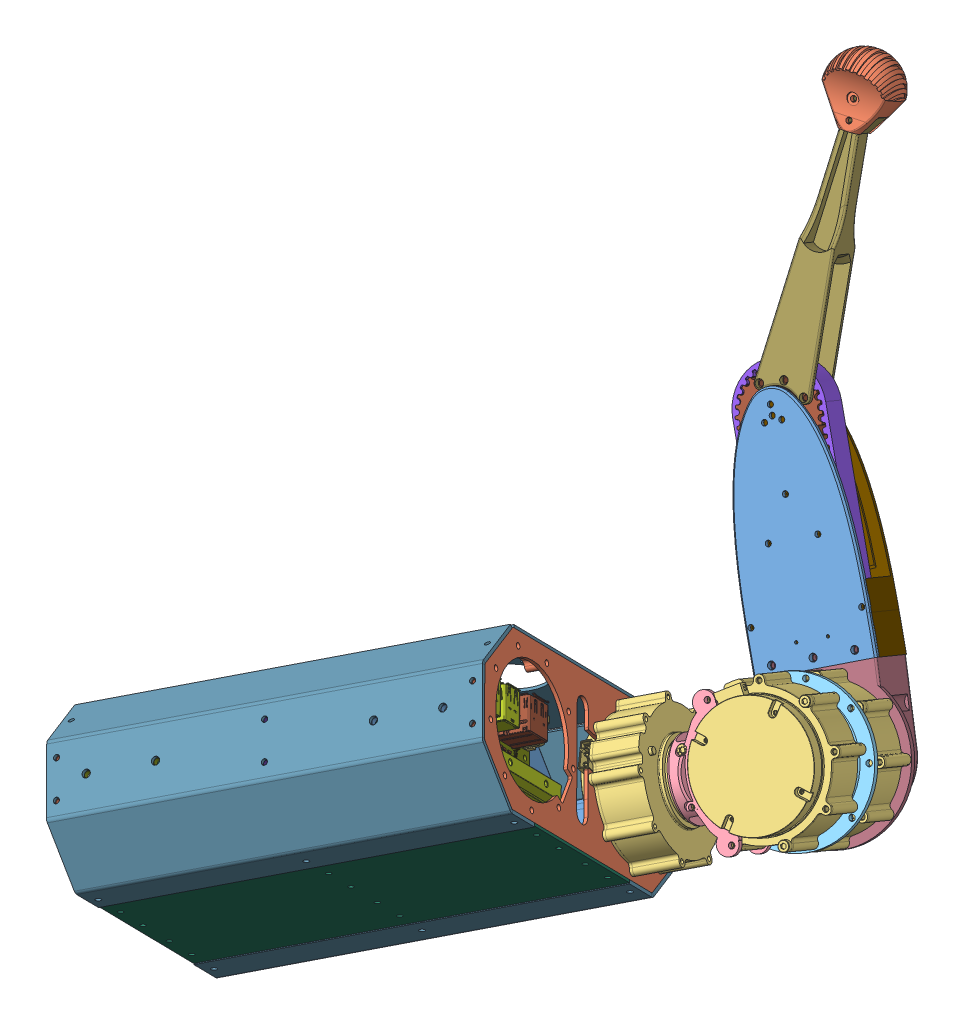
SolidWorks assembly OpenPaws, configuration 默认. Lengths in mm. (continued)
Components (placement in the parent): (continued)
- Jetson nano.step-1: Jetson nano.step [默认] at (68.0286 -15.5875 328.1241) x (0.005778 0.713341 0.700793) z (0.818097 0.399633 -0.413534) size (100 81.03 30.51) (continued)
  - 142-13449-1000-A02_ASM.step-1: 142-13449-1000-A02_ASM.step [默认] at origin size (100 81.03 23.18) (continued)
    - 1206_H190.step-1: 1206_H190.step [默认] at (82 18.8 1.575) x (0 1 0) z (0 0 1) size (3.2 1.6 1.9)
    - 1206_H190.step-2: 1206_H190.step [默认] at (81.95 13.5 1.575) x (0 -1 0) z (0 0 1) size (3.2 1.6 1.9)
    - 300-0868-000_3.step-1: 300-0868-000_3.step [默认] at (69.6 4 1.575) x (-1 0 0) z (0 0 1) size (1 0.6 0.4)
    - 300-0868-000_3.step-2: 300-0868-000_3.step [默认] at (9.55 0.95 1.575) size (1 0.6 0.4)
    - 300-0868-000_3.step-3: 300-0868-000_3.step [默认] at (19.6 31.45 1.575) x (0 -1 0) z (0 0 1) size (1 0.6 0.4)
    - 300-0868-000_3.step-4: 300-0868-000_3.step [默认] at (91.45 -2.45 1.575) x (-1 0 0) z (0 0 1) size (1 0.6 0.4)
    - 300-0868-000_3.step-5: 300-0868-000_3.step [默认] at (84.6 -5.1 1.575) size (1 0.6 0.4)
    - 300-0868-000_3.step-6: 300-0868-000_3.step [默认] at (66.725 5.875 1.575) x (0 -1 0) z (0 0 1) size (1 0.6 0.4)
    - 300-0868-000_3.step-7: 300-0868-000_3.step [默认] at (20.8 31.45 1.575) x (0 -1 0) z (0 0 1) size (1 0.6 0.4)
    - 300-0868-000_3.step-8: 300-0868-000_3.step [默认] at (62.9 31.35 1.575) x (-1 0 0) z (0 0 1) size (1 0.6 0.4)
    - 300-0868-000_3.step-9: 300-0868-000_3.step [默认] at (65.475 4.8 1.575) x (-1 0 0) z (0 0 1) size (1 0.6 0.4)
    - 300-0868-000_3.step-10: 300-0868-000_3.step [默认] at (63.9 33.85 1.575) x (-1 0 0) z (0 0 1) size (1 0.6 0.4)
    - 300-0868-000_3.step-11: 300-0868-000_3.step [默认] at (15.65 27.9 1.575) size (1 0.6 0.4)
    - 300-0868-000_3.step-12: 300-0868-000_3.step [默认] at (11.8 6.1 1.575) x (0 1 0) z (0 0 1) size (1 0.6 0.4)
    - 300-0868-000_3.step-13: 300-0868-000_3.step [默认] at (22.1 6.25 1.575) x (0 1 0) z (0 0 1) size (1 0.6 0.4)
    - 300-0869-000_3.step-1: 300-0869-000_3.step [默认] at (9.65 8.1 1.575) x (0 -1 0) z (0 0 1) size (1 0.6 0.53)
    - 300-0402-000_1.step-1: 300-0402-000_1.step [默认] at (20.8 26.45 1.575) x (0 -1 0) z (0 0 1) size (2 2.69 1.1)
    - 300-0560-000_1.step-1: 300-0560-000_1.step [默认] at (6.8 43.65 1.575) x (-1 0 0) z (0 0 1) size (2 2.69 1.1)
    - 174-0159-000_2.step-1: 174-0159-000_2.step [默认] at (61.49 57.15 1.575) x (-1 0 0) z (0 0 1) size (2 3.52 0.6)
    - 064-0373-000_2.step-1: 064-0373-000_2.step [默认] at (72.95 -7.825 1.575) size (17.8 21.6 17.45)
    - 064-0375-000_2.step-1: 064-0375-000_2.step [默认] at (19.751 -12.275 1.575) size (16.2 5.58 0.01)
    - 074-0221-000_3.step-1: 074-0221-000_3.step [默认] at (86 29 1.575) x (0 1 0) z (0 0 1) size (50.8 5.08 11.6)
    - 2016MM_H100.step-1: 2016MM_H100.step [默认] at (24.5 49.25 1.575) x (0 1 0) z (0 0 1) size (2 1.6 1)
    - 065-0656-000_2.step-1: 065-0656-000_2.step [默认] at (55.6 -10.04 1.575) x (-1 0 0) z (0 0 1) size (16.19 17.45 19.62)
    - 065-0656-000_2.step-2: 065-0656-000_2.step [默认] at (38.6 -10.04 1.575) x (-1 0 0) z (0 0 1) size (16.19 17.45 19.62)
    - 115-1921-000_3.step-1: 115-1921-000_3.step [默认] at (80.45 50.52 1.575) x (0 -1 0) z (0 0 1) size (5 4 1)
    - 115-1921-000_3.step-2: 115-1921-000_3.step [默认] at (80.4 34.5 1.575) x (0 -1 0) z (0 0 1) size (5 4 1)
    - 115-1921-000_3.step-3: 115-1921-000_3.step [默认] at (77.2 25.9 1.575) x (0 -1 0) z (0 0 1) size (5 4 1)
    - 085-0328-000_2.step-1: 085-0328-000_2.step [默认] at (16.28 36.32 1.575) x (0 -1 0) z (0 0 1) size (3.81 2.5 0.6)
    - 074-0216-000_2.step-1: 074-0216-000_2.step [默认] at (92.14 58 1.575) x (-1 0 0) z (0 0 1) size (4.83 5 11.5)
    - 060-0002-000_1.step-1: 060-0002-000_1.step [默认] at (41.2 57.9 1.575) x (0 -1 0) z (0 0 1) size (5.1 5.4 1.68)
    - 316-0697-000_1.step-1: 316-0697-000_1.step [默认] at (50.6 58.1 1.575) x (0 -1 0) z (0 0 1) size (3 3.72 0.8)
    - 032-0256-000_1.step-1: 032-0256-000_1.step [默认] at (5.925 9.425 1.575) size (4.22 2.82 2)
    - 041-0092-000_1.step-1: 041-0092-000_1.step [默认] at (46.9 54.9 1.575) x (0 -1 0) z (0 0 1) size (4.22 2.82 1.2)
    - 080-1243-000_3.step-1: 080-1243-000_3.step [默认] at (69.9 40.3 1.575) x (0 -1 0) z (0 0 1) size (21.9 9.1 4.8)
    - 102-0066-000_2.step-1: 102-0066-000_2.step [默认] at (18 4.2 1.575) size (1 1.86 0.61)
    - 102-0066-000_2.step-2: 102-0066-000_2.step [默认] at (13.55 4.2 1.575) size (1 1.86 0.61)
    - 102-0066-000_2.step-3: 102-0066-000_2.step [默认] at (32.45 5.81 1.575) size (1 1.86 0.61)
    - 102-0066-000_2.step-4: 102-0066-000_2.step [默认] at (27.65 5.81 1.575) size (1 1.86 0.61)
    - 102-0066-000_2.step-5: 102-0066-000_2.step [默认] at (20.15 4.2 1.575) size (1 1.86 0.61)
    - 102-0066-000_2.step-6: 102-0066-000_2.step [默认] at (15.75 4.2 1.575) size (1 1.86 0.61)
    - 102-0066-000_2.step-7: 102-0066-000_2.step [默认] at (29.25 5.81 1.575) size (1 1.86 0.61)
    - 102-0066-000_2.step-8: 102-0066-000_2.step [默认] at (30.85 5.81 1.575) size (1 1.86 0.61)
    - 102-0037-000_1.step-1: 102-0037-000_1.step [默认] at (55.2 2.95 1.575) x (-1 0 0) z (0 0 1) size (1 1.86 0.91)
    - 102-0037-000_1.step-2: 102-0037-000_1.step [默认] at (39.99 2.87 1.575) x (-1 0 0) z (0 0 1) size (1 1.86 0.91)
    - 102-0037-000_1.step-3: 102-0037-000_1.step [默认] at (60.55 2.95 1.575) x (-1 0 0) z (0 0 1) size (1 1.86 0.91)
    - 102-0037-000_1.step-4: 102-0037-000_1.step [默认] at (38.22 2.87 1.575) x (-1 0 0) z (0 0 1) size (1 1.86 0.91)
    - 0805_H140.step-1: 0805_H140.step [默认] at (8.1 -2.1 1.575) size (2.01 1.25 1.4)
    - 0805_H150.step-1: 0805_H150.step [默认] at (82.9 -8.4 1.575) x (-1 0 0) z (0 0 1) size (2.01 1.25 1.5)
    - 0603_H100.step-1: 0603_H100.step [默认] at (6.1 41.525 1.575) x (-1 0 0) z (0 0 1) size (1.6 0.81 1)
    - 0603_H060.step-1: 0603_H060.step [默认] at (63.25 -12 1.575) x (0 1 0) z (0 0 1) size (1.6 0.81 0.6)
    - 0603_H060.step-2: 0603_H060.step [默认] at (63.8 -0.7 1.575) x (0 -1 0) z (0 0 1) size (1.6 0.81 0.6)
    - 0603_H060.step-3: 0603_H060.step [默认] at (82.4 -10 1.575) x (-1 0 0) z (0 0 1) size (1.6 0.81 0.6)
    - 0603_H100.step-2: 0603_H100.step [默认] at (9.486 -7.5 1.575) x (-1 0 0) z (0 0 1) size (1.6 0.81 1)
    - 0603_H100.step-3: 0603_H100.step [默认] at (17.4 57.4 1.575) x (0 -1 0) z (0 0 1) size (1.6 0.81 1)
    - 0603_H100.step-4: 0603_H100.step [默认] at (30.35 25.9 1.575) x (0 -1 0) z (0 0 1) size (1.6 0.81 1)
    - 0603_H100.step-5: 0603_H100.step [默认] at (11.4 45.7 1.575) size (1.6 0.81 1)
    - 0603_H100.step-6: 0603_H100.step [默认] at (3.2 43 1.575) size (1.6 0.81 1)
    - 0603_H100.step-7: 0603_H100.step [默认] at (74.7 53.4 1.575) x (0 -1 0) z (0 0 1) size (1.6 0.81 1)
    - 0603_H100.step-8: 0603_H100.step [默认] at (69.5 53.9 1.575) x (0 -1 0) z (0 0 1) size (1.6 0.81 1)
    - 0603_H100.step-9: 0603_H100.step [默认] at (52.5 52.9 1.575) x (-1 0 0) z (0 0 1) size (1.6 0.81 1)
    - 0603_H100.step-10: 0603_H100.step [默认] at (52.5 54.2 1.575) x (-1 0 0) z (0 0 1) size (1.6 0.81 1)
    - 0603_H100.step-11: 0603_H100.step [默认] at (27.3 51.35 1.575) size (1.6 0.81 1)
    - 0603_H100.step-12: 0603_H100.step [默认] at (22.7 49.1 1.575) x (0 1 0) z (0 0 1) size (1.6 0.81 1)
    - 0603_H100.step-13: 0603_H100.step [默认] at (26.2 48.8 1.575) x (0 1 0) z (0 0 1) size (1.6 0.81 1)
    - 0603_H100.step-14: 0603_H100.step [默认] at (20.9 49.1 1.575) x (0 1 0) z (0 0 1) size (1.6 0.81 1)
    - 0603_H100.step-15: 0603_H100.step [默认] at (65.5 27.4 1.575) x (0 -1 0) z (0 0 1) size (1.6 0.81 1)
    - 0603_H100.step-16: 0603_H100.step [默认] at (63.8 52.2 1.575) x (-1 0 0) z (0 0 1) size (1.6 0.81 1)
    - 0603_H100.step-17: 0603_H100.step [默认] at (52.5 55.4 1.575) x (-1 0 0) z (0 0 1) size (1.6 0.81 1)
    - 080-1669-000_2.step-1: 080-1669-000_2.step [默认] at (0.2 29 1.575) x (0 -1 0) z (0 0 1) size (22.4 5.4 7.7)
  - 244-63448-0000-000_ASM.step-1: 244-63448-0000-000_ASM.step [默认] at (11.2 22.5 8.2712) size (69.6 45 21.37)
    - 142-13448-1000-A02_ASM.step-1: 142-13448-1000-A02_ASM.step [默认] at origin size (23 37.01 4.01)
      - 080-0051-000_3.step-1: 080-0051-000_3.step [默认] at (28.331 29.139 0) x (-1 0 0) z (0 0 -1) size (13.4 17 1.28)
      - TM670M-A2_1.step-1: TM670M-A2_1.step [默认] at (23.7 13.45 1.2) size (23 23 1.29)
    - 142-13448-1000-A02-SKU0000_ASM.step-1: 142-13448-1000-A02-SKU0000_ASM.step [默认] at origin size (23 23 1.29)
      - TM670M-A2_1.step-1: TM670M-A2_1.step [默认] at (23.7 13.45 1.2) size (23 23 1.29)
    - PORG_HSK_ASSY_ASM.step-1: PORG_HSK_ASSY_ASM.step [默认] at (0 0 4.01) size (58.7 39.4 17.3)
      - PORG_HEAT_SINK.step-1: PORG_HEAT_SINK.step [默认] at origin size (58.7 39.4 17.3)
    - 142-63448-1GEN_A00.step-1: 142-63448-1GEN_A00.step [默认] at origin size (69.6 45 1.2)
    - PORG_LEAF_SPRING_DRAWN.step-1: PORG_LEAF_SPRING_DRAWN.step [默认] at (0 0 -0.4) x (1 0.000001 0) z (0 0 1) size (39.83 21.3 1.2)
    - PORG_LEAF_SPRING_SCREW.step-1: PORG_LEAF_SPRING_SCREW.step [默认] at (6.9871 5.9982 5.21) x (0 0 -1) z (0 1 0) size (6.41 4.7 4.7)
    - PORG_LEAF_SPRING_SCREW.step-2: PORG_LEAF_SPRING_SCREW.step [默认] at (6.9871 20.9018 5.21) x (0 0 -1) z (0 1 0) size (6.41 4.7 4.7)
    - PORG_LEAF_SPRING_SCREW.step-3: PORG_LEAF_SPRING_SCREW.step [默认] at (40.4129 20.9018 5.21) x (0 0 -1) z (0 1 0) size (6.41 4.7 4.7)
    - PORG_LEAF_SPRING_SCREW.step-4: PORG_LEAF_SPRING_SCREW.step [默认] at (40.4129 5.9982 5.21) x (0 0 -1) z (0 1 0) size (6.41 4.7 4.7)
  - PORG_HEX_STANDOFF.step-1: PORG_HEX_STANDOFF.step [默认] at (75.8 58.5 8.17) x (-1 0 0) z (0 0 -1) size (5.14 4.45 6.57)
  - PORG_HEX_STANDOFF.step-2: PORG_HEX_STANDOFF.step [默认] at (12.2 58.5 8.17) x (-1 0 0) z (0 0 -1) size (5.14 4.45 6.57)
  - PORG_SYSTEM_SCREW.step-1: PORG_SYSTEM_SCREW.step [默认] at (12.2 58.5 3.73) size (4.55 4.55 4.53)
  - PORG_SYSTEM_SCREW.step-2: PORG_SYSTEM_SCREW.step [默认] at (75.8 58.5 3.73) size (4.55 4.55 4.53)
  - PORG_SYSTEM_SCREW.step-3: PORG_SYSTEM_SCREW.step [默认] at (75.8 58.5 5.67) x (-1 0 0) z (0 0 -1) size (4.55 4.55 4.53)
  - PORG_SYSTEM_SCREW.step-4: PORG_SYSTEM_SCREW.step [默认] at (12.2 58.5 5.67) x (-1 0 0) z (0 0 -1) size (4.55 4.55 4.53)
  - 155-0576-000.step-1: 155-0576-000.step [默认] at (40.276 40.3 5.01) size (5 5 4.08)
- BottomSidePanel-2: BottomSidePanel [默认] at (48.6942 34.1994 363.8747) x (-0.818097 -0.399633 0.413534) z (-0.005778 -0.713341 -0.700793) size (220 1.5 123.55)
- Battery6S-1: Battery6S [默认] at (15.3803 -38.1785 419.7744) x (0.818097 0.399633 -0.413534) z (0.005778 0.713341 0.700793) size (130 50 100)
- FrontFrame-2: FrontFrame [默认] at (0.2435 -6.3072 444.8108) x (-0.005778 -0.713341 -0.700793) z (-0.575051 0.575706 -0.581273) size (175.11 55 85)
- MiddleFrame-1: MiddleFrame [默认] at (32.4476 -54.4826 365.2373) x (0.005778 0.713341 0.700793) z (-0.575051 0.575706 -0.581273) size (175 10 85)
- UpperLink-1: UpperLink [默认] at (120.9392 35.0483 197.2427) x (-0.816621 -0.40178 0.414372) z (-0.540637 0.783855 -0.305422) size (62 27.01 125.98)
- UpperLinkCover-1: UpperLinkCover [默认] at (139.9453 55.47 216.0109) x (0.816621 0.40178 -0.414372) z (-0.540637 0.783855 -0.305422) size (62 3.5 126)
- Foot-1: Foot [默认] at (68.3392 238.7706 115.6756) x (0.970121 0.023224 -0.241508) z (-0.202095 -0.473439 -0.857329) size (38.01 39.33 33.29)
Mates (geometry in assembly coordinates):
- 平行8: parallel anti-aligned: plane of Shoulder-1 through (126.526 -8.5635 317.638) normal (0.818097 0.399633 -0.413534); plane of GearMotor-2 through (119.5722 -11.9604 321.1531) normal (-0.818097 -0.399633 0.413534)
- 重合24: coincident aligned: circle of Shoulder-1; circle of GearMotor-2
- 同心28: concentric aligned: circle of Shoulder-1; circle of GearMotor-2
- 重合25: coincident anti-aligned: plane of Shoulder-1 through (126.526 -8.5635 317.638) normal (0.818097 0.399633 -0.413534); plane of GearMotor-2 through (126.526 -8.5635 317.638) normal (-0.818097 -0.399633 0.413534)
- 平行9: parallel anti-aligned: plane of GearMotor-2 through (149.4328 2.6262 306.0591) normal (0.818097 0.399633 -0.413534); plane of ShoulderConnector-1 through (183.3692 -58.8329 313.8026) normal (-0.818097 -0.399633 0.413534)
- 同心29: concentric anti-aligned: circle of GearMotor-2; circle of ShoulderConnector-1
- 同心30: concentric anti-aligned: circle of GearMotor-2; circle of ShoulderConnector-1
- 重合26: coincident anti-aligned: plane of GearMotor-2 through (149.4328 2.6262 306.0591) normal (0.818097 0.399633 -0.413534); plane of ShoulderConnector-1 through (183.3692 -58.8329 313.8026) normal (-0.818097 -0.399633 0.413534)
- 平行10: parallel anti-aligned: plane of ShoulderConnector-1 through (211.9927 -34.2835 326.3914) normal (-0.202095 -0.473439 -0.857329); plane of GearMotor-3 through (188.7302 29.7295 306.4399) normal (0.202095 0.473439 0.857329)
- 重合27: coincident anti-aligned: plane of ShoulderConnector-1 through (211.9927 -34.2835 326.3914) normal (-0.202095 -0.473439 -0.857329); plane of GearMotor-3 through (187.0124 25.7053 299.1526) normal (0.202095 0.473439 0.857329)
- 平行11: parallel anti-aligned: plane of GearMotor-3 through (181.3538 12.449 275.1473) normal (-0.202095 -0.473439 -0.857329); plane of ConnectorPlate-1 through (180.5751 12.35 275.3856) normal (0.202095 0.473439 0.857329)
- 同心37: concentric aligned: circle of GearMotor-3; circle of ConnectorPlate-1
- 同心38: concentric aligned: circle of GearMotor-3; circle of ConnectorPlate-1
- 重合29: coincident anti-aligned: plane of GearMotor-3 through (181.3538 12.449 275.1473) normal (-0.202095 -0.473439 -0.857329); plane of ConnectorPlate-1 through (180.5751 12.35 275.3856) normal (0.202095 0.473439 0.857329)
- 同心39: concentric anti-aligned: cylinder of ConnectorPlate-1 through (178.6255 6.0576 263.5734) axis (0.202095 0.473439 0.857329) radius 33; cylinder of GearMotor-6 through (178.4173 5.5699 262.6903) axis (-0.202095 -0.473439 -0.857329) radius 35.5
- 重合30: coincident anti-aligned: plane of ConnectorPlate-1 through (179.5647 9.9828 271.0989) normal (-0.202095 -0.473439 -0.857329); plane of GearMotor-6 through (180.3433 10.0818 270.8607) normal (0.202095 0.473439 0.857329)
- 同心40: concentric anti-aligned: circle of ConnectorPlate-1; circle of GearMotor-6
- 同心42: concentric aligned: circle of GearMotor-6; circle of WheelGuard-1
- 同心43: concentric aligned: circle of GearMotor-6; circle of WheelGuard-1
- 重合31: coincident anti-aligned: plane of GearMotor-6 through (172.9668 -7.1987 239.5682) normal (-0.202095 -0.473439 -0.857329); plane of WheelGuard-1 through (172.9668 -7.1987 239.5682) normal (0.202095 0.473439 0.857329)
- 同心44: concentric aligned: circle of WheelGuard-1; circle of Wheel-1
- 同心45: concentric aligned: circle of WheelGuard-1; circle of Wheel-1
- 重合32: coincident anti-aligned: plane of WheelGuard-1 through (172.1585 -9.0925 236.1389) normal (-0.202095 -0.473439 -0.857329); plane of Wheel-1 through (189.4159 -21.1677 238.7391) normal (0.202095 0.473439 0.857329)
- 同心46: concentric anti-aligned: circle of Wheel-1; circle of WheelGuard-2
- 同心47: concentric anti-aligned: circle of Wheel-1; circle of WheelGuard-2
- 重合34: coincident anti-aligned: plane of Wheel-1 through (186.3845 -28.2693 225.8791) normal (-0.202095 -0.473439 -0.857329); plane of WheelGuard-2 through (169.127 -16.194 223.2789) normal (0.202095 0.473439 0.857329)
- 同心67: concentric aligned: circle of KneePivot-1; circle of Bearing-1
- 同心69: concentric aligned: circle of KneePivot-1; circle of Bearing-2
- 同心70: concentric anti-aligned: circle of KneePivot-1; circle of KneeWheel-1
- 同心73: concentric aligned: circle of KneeWheel-1; circle of LowerLeg-1
- 同心74: concentric anti-aligned: circle of KneeWheel-1; circle of LowerLeg-1
- 平行12: parallel anti-aligned: line of Shoulder-1 through (93.8085 -0.0591 285.313) axis (0.005778 0.713341 0.700793); line of Shoulder-2 through (-69.097 8.1485 454.6038) axis (-0.005778 -0.713341 -0.700793)
- 同心82: concentric aligned: cylinder of Shoulder-1 through (104.9805 -14.6979 281.177) axis (-0.410708 -0.097322 -0.906558) radius 1.25; cylinder of Side Panel-1 through (108.2644 -13.9197 288.4258) axis (-0.410708 -0.097322 -0.906558) radius 1.5
- 同心83: concentric aligned: cylinder of Shoulder-1 through (116.4395 -35.1216 284.1093) axis (-0.005778 -0.713341 -0.700793) radius 1.25; cylinder of Side Panel-1 through (116.4394 -35.1257 284.1052) axis (-0.005778 -0.713341 -0.700793) radius 1.55
- 锁定1: lock: unknown of BackFrame-1; unknown of Side Panel-1
- 同心84: concentric anti-aligned: cylinder of BackFrame-1 through (109.6874 -75.4068 268.0933) axis (0.005778 0.713341 0.700793) radius 2; cylinder of Side Panel-1 through (109.9185 -46.8773 296.121) axis (-0.005778 -0.713341 -0.700793) radius 2.1
- 同心86: concentric anti-aligned: cylinder of Shoulder-1 through (147.3189 19.738 398.2137) axis (0.575051 -0.575706 0.581273) radius 1.25; cylinder of TopSidePanel-1 through (153.0694 13.981 404.0264) axis (-0.575051 0.575706 -0.581273) radius 1.5
- 平行13: parallel anti-aligned: cylinder of Shoulder-1 through (147.0672 -11.3289 367.6932) axis (0.575051 -0.575706 0.581273) radius 1.25; cylinder of TopSidePanel-1 through (152.8178 -17.0779 373.5139) axis (-0.575051 0.575706 -0.581273) radius 1.5
- 平行14: parallel anti-aligned: cylinder of Shoulder-1 through (146.9517 -25.5957 353.6773) axis (0.575051 -0.575706 0.581273) radius 1.25; cylinder of TopSidePanel-1 through (152.7022 -31.3447 359.498) axis (-0.575051 0.575706 -0.581273) radius 1.5
- 同心89: concentric anti-aligned: cylinder of Shoulder-1 through (147.2033 5.4712 384.1978) axis (0.575051 -0.575706 0.581273) radius 1.25; cylinder of TopSidePanel-1 through (152.9538 -0.2858 390.0105) axis (-0.575051 0.575706 -0.581273) radius 1.5
- 重合46: coincident anti-aligned: plane of Shoulder-1 through (142.7848 -37.0273 346.4775) normal (0.575051 -0.575706 0.581273); plane of TopSidePanel-1 through (25.0074 -61.3631 438.8915) normal (-0.575051 0.575706 -0.581273)
- 同心90: concentric aligned: cylinder of Shoulder-1 through (147.4344 34.0049 412.2295) axis (0.575051 -0.575706 0.581273) radius 1.25; cylinder of Side Panel-2 through (147.4368 34.0025 412.232) axis (0.575051 -0.575706 0.581273) radius 1.6
- 同心91: concentric aligned: cylinder of Shoulder-1 through (105.8478 92.3775 386.3689) axis (-0.402537 0.911494 0.084514) radius 1.25; cylinder of Side Panel-2 through (109.0688 85.0839 385.6927) axis (-0.402537 0.911494 0.084514) radius 1.5
- 同心92: concentric anti-aligned: cylinder of BackFrame-1 through (68.5255 45.7598 388.3923) axis (-0.818097 -0.399633 0.413534) radius 1.5; cylinder of Jetson nano.step-1/142-13449-1000-A02_ASM.step-1/142-13449-1000-A02.step-1 through (68.5255 45.7598 388.3923) axis (0.818097 0.399633 -0.413534) radius 1.375
- 同心93: concentric anti-aligned: cylinder of BackFrame-1 through (68.0286 -15.5875 328.1241) axis (-0.818097 -0.399633 0.413534) radius 1.5; cylinder of Jetson nano.step-1/142-13449-1000-A02_ASM.step-1/142-13449-1000-A02.step-1 through (68.0286 -15.5875 328.1241) axis (0.818097 0.399633 -0.413534) radius 1.375
- 重合47: coincident anti-aligned: plane of BackFrame-1 through (68.5255 45.7598 388.3923) normal (0.818097 0.399633 -0.413534); plane of Jetson nano.step-1/142-13449-1000-A02_ASM.step-1/142-13449-1000-A02.step-1 through (68.0286 -15.5875 328.1241) normal (-0.818097 -0.399633 0.413534)
- 同心94: concentric aligned: cylinder of Shoulder-1 through (98.0723 23.3393 304.2691) axis (-0.575051 0.575706 -0.581273) radius 1.25; cylinder of BottomSidePanel-2 through (102.9602 18.4458 309.21) axis (-0.575051 0.575706 -0.581273) radius 1.5
- 平行16: parallel anti-aligned: line of Shoulder-1 through (101.9894 3.9373 281.1777) axis (0.005778 0.713341 0.700793); line of BottomSidePanel-2 through (101.8408 92.9341 366.8888) axis (-0.005778 -0.713341 -0.700793)
- 重合48: coincident anti-aligned: plane of Shoulder-1 through (93.9054 11.9077 297.0693) normal (-0.575051 0.575706 -0.581273); plane of BottomSidePanel-2 through (48.6942 34.1994 363.8747) normal (0.575051 -0.575706 0.581273)
- 同心97: concentric anti-aligned: cylinder of ShoulderConnector-1 through (189.7643 -5.8599 319.4342) axis (-0.202095 -0.473439 -0.857329) radius 1.6; cylinder of GearMotor-3 through (189.1577 -7.2799 316.8621) axis (0.202095 0.473439 0.857329) radius 1.55
- 同心98: concentric aligned: cylinder of ShoulderConnector-1 through (154.7941 45.1242 299.5229) axis (-0.202095 -0.473439 -0.857329) radius 1.6; cylinder of GearMotor-3 through (153.9797 43.2162 296.0679) axis (-0.202095 -0.473439 -0.857329) radius 1.25
- 同心105: concentric aligned: cylinder of Shoulder-2 through (-24.3659 -49.9181 499.0717) axis (0.575051 -0.575706 0.581273) radius 1.25; cylinder of Side Panel-2 through (-24.3635 -49.9205 499.0742) axis (0.575051 -0.575706 0.581273) radius 1.6
- 平行20: parallel aligned: cylinder of Shoulder-2 through (-24.9643 -123.7855 426.5037) axis (0.575051 -0.575706 0.581273) radius 1.25; cylinder of Side Panel-1 through (-24.9643 -123.7885 426.5007) axis (0.575051 -0.575706 0.581273) radius 1.6
- 重合51: coincident anti-aligned: plane of Shoulder-2 through (-20.3146 -52.7533 492.2557) normal (0.575051 -0.575706 0.581273); plane of TopSidePanel-1 through (25.0074 -61.3631 438.8915) normal (-0.575051 0.575706 -0.581273)
- 平行24: parallel anti-aligned: plane of Shoulder-2 through (-51.2991 -31.4828 470.8599) normal (0.818097 0.399633 -0.413534); plane of Battery6S-1 through (-66.5485 -35.3693 417.5905) normal (-0.818097 -0.399633 0.413534)
- 重合58: coincident anti-aligned: plane of Shoulder-2 through (-44.7543 -28.2858 467.5516) normal (0.818097 0.399633 -0.413534); plane of Battery6S-1 through (-66.5485 -35.3693 417.5905) normal (-0.818097 -0.399633 0.413534)
- 同心110: concentric aligned: cylinder of Side Panel-2 through (-7.6919 20.0134 478.7298) axis (0.005778 0.713341 0.700793) radius 2.1; cylinder of FrontFrame-2 through (-8.9343 -133.3549 328.0593) axis (0.005778 0.713341 0.700793) radius 2
- 同心111: concentric aligned: cylinder of Side Panel-2 through (-36.3253 6.0263 493.2035) axis (0.005778 0.713341 0.700793) radius 2.1; cylinder of FrontFrame-2 through (-37.5676 -147.3421 342.533) axis (0.005778 0.713341 0.700793) radius 2
- 重合59: coincident anti-aligned: plane of Side Panel-2 through (117.1708 96.0877 400.2639) normal (-0.005778 -0.713341 -0.700793); plane of FrontFrame-2 through (-3.6014 22.0116 476.6622) normal (0.005778 0.713341 0.700793)
- 重合63: coincident anti-aligned: plane of GearMotor-6 through (174.0626 -5.2559 241.7363) normal (-0.202095 -0.473439 -0.857329); plane of ThighRoot-2 through (236.5323 -46.6268 249.8566) normal (0.202095 0.473439 0.857329)
- 同心135: concentric aligned: cylinder of ThighRoot-2 through (126.6389 8.2749 213.9501) axis (-0.202095 -0.473439 -0.857329) radius 1.65; cylinder of FrontThigh-1 through (126.6793 8.3696 214.1215) axis (-0.202095 -0.473439 -0.857329) radius 1.5
- 同心136: concentric aligned: cylinder of ThighRoot-2 through (143.7879 16.7122 205.2483) axis (-0.202095 -0.473439 -0.857329) radius 1.65; cylinder of FrontThigh-1 through (143.8283 16.8069 205.4197) axis (-0.202095 -0.473439 -0.857329) radius 1.5
- 同心137: concentric anti-aligned: cylinder of ThighRoot-2 through (160.9369 25.1496 196.5465) axis (-0.202095 -0.473439 -0.857329) radius 1.65; cylinder of 11FrontThighCover4-1 through (165.7468 36.4175 216.9509) axis (0.202095 0.473439 0.857329) radius 2
- 同心138: concentric anti-aligned: cylinder of ThighRoot-2 through (143.7879 16.7122 205.2483) axis (-0.202095 -0.473439 -0.857329) radius 1.65; cylinder of 11FrontThighCover4-1 through (148.5978 27.9801 225.6527) axis (0.202095 0.473439 0.857329) radius 2
- 重合65: coincident anti-aligned: plane of ThighRoot-2 through (130.9531 14.0496 237.5048) normal (0.202095 0.473439 0.857329); plane of 11FrontThighCover4-1 through (139.339 54.0497 213.4389) normal (-0.202095 -0.473439 -0.857329)
- 同心139: concentric aligned: cylinder of KneePivot-1 through (90.331 112.9224 193.1849) axis (0.202095 0.473439 0.857329) radius 1.65; cylinder of 11FrontThighCover4-1 through (90.411 113.1099 193.5245) axis (0.202095 0.473439 0.857329) radius 1.5
- 同心140: concentric aligned: cylinder of KneePivot-1 through (87.6278 116.8416 191.6578) axis (0.202095 0.473439 0.857329) radius 1.65; cylinder of 11FrontThighCover4-1 through (87.7078 117.0291 191.9973) axis (0.202095 0.473439 0.857329) radius 1.5
- 同心141: concentric anti-aligned: cylinder of KneePivot-1 through (84.6723 99.6661 169.1797) axis (0.202095 0.473439 0.857329) radius 8.4; cylinder of KneeWheel-1 through (89.5602 111.1167 189.915) axis (-0.202095 -0.473439 -0.857329) radius 10.5
- 重合80: coincident anti-aligned: plane of ThighRoot-2 through (166.8794 22.8989 196.6219) normal (-0.202095 -0.473439 -0.857329); plane of FrontThigh-1 through (121.5454 36.4686 199.8147) normal (0.202095 0.473439 0.857329)
- 重合81: coincident anti-aligned: plane of Bearing-2 through (85.4395 101.4633 172.4342) normal (-0.202095 -0.473439 -0.857329); plane of FrontThigh-1 through (121.5454 36.4686 199.8147) normal (0.202095 0.473439 0.857329)
- 重合86: coincident anti-aligned: plane of Bearing-1 through (90.31 112.8731 193.0958) normal (0.202095 0.473439 0.857329); plane of 11FrontThighCover4-1 through (90.31 112.8731 193.0958) normal (-0.202095 -0.473439 -0.857329)
- 同心142: concentric anti-aligned: cylinder of Wheel-1 through (172.1686 -9.0713 236.1248) axis (-0.202095 -0.473439 -0.857329) radius 7.5; cylinder of Belt-1 through (170.6529 -12.6221 229.6948) axis (0.202095 0.473439 0.857329) radius 23.448
- 重合87: coincident aligned: plane of Wheel-1 through (186.3845 -28.2693 225.8791) normal (-0.202095 -0.473439 -0.857329); plane of Belt-1 through (149.9665 -25.561 232.9682) normal (-0.202095 -0.473439 -0.857329)
- 同心143: concentric aligned: cylinder of KneeWheel-1 through (87.4122 125.205 182.6414) axis (0.202095 0.473439 0.857329) radius 1.65; cylinder of LowerLeg-1 through (77.9137 102.9534 142.347) axis (0.202095 0.473439 0.857329) radius 2.1
- 同心144: concentric aligned: cylinder of KneeWheel-1 through (87.4122 125.205 182.6414) axis (0.202095 0.473439 0.857329) radius 1.65; cylinder of LowerLeg-1 through (77.9137 102.9534 142.347) axis (0.202095 0.473439 0.857329) radius 2.1
- 重合88: coincident anti-aligned: plane of KneeWheel-1 through (86.3183 122.5842 166.8504) normal (-0.202095 -0.473439 -0.857329); plane of LowerLeg-1 through (77.7354 161.6892 147.2788) normal (0.202095 0.473439 0.857329)
- 重合89: coincident anti-aligned: plane of Battery6S-1 through (-13.3722 -9.3932 390.7108) normal (-0.575051 0.575706 -0.581273); plane of FrontFrame-2 through (-25.4114 13.2836 425.0807) normal (0.575051 -0.575706 0.581273)
- 重合101: coincident anti-aligned: plane of LowerLeg-1 through (75.1105 233.3221 122.9203) normal (-0.13425 0.880521 -0.454599); plane of Paw-1 through (69.5475 230.8459 119.767) normal (0.13425 -0.880521 0.454599)
- 重合102: coincident anti-aligned: plane of LowerLeg-1 through (78.2406 162.8728 149.4222) normal (-0.202095 -0.473439 -0.857329); plane of Paw-1 through (49.1346 228.0142 120.3105) normal (0.202095 0.473439 0.857329)
- 同心145: concentric anti-aligned: circle of Side Panel-2; circle of MiddleFrame-1
- 同心146: concentric aligned: circle of Side Panel-2; circle of MiddleFrame-1
- 同心147: concentric aligned: circle of Side Panel-2; circle of MiddleFrame-1
